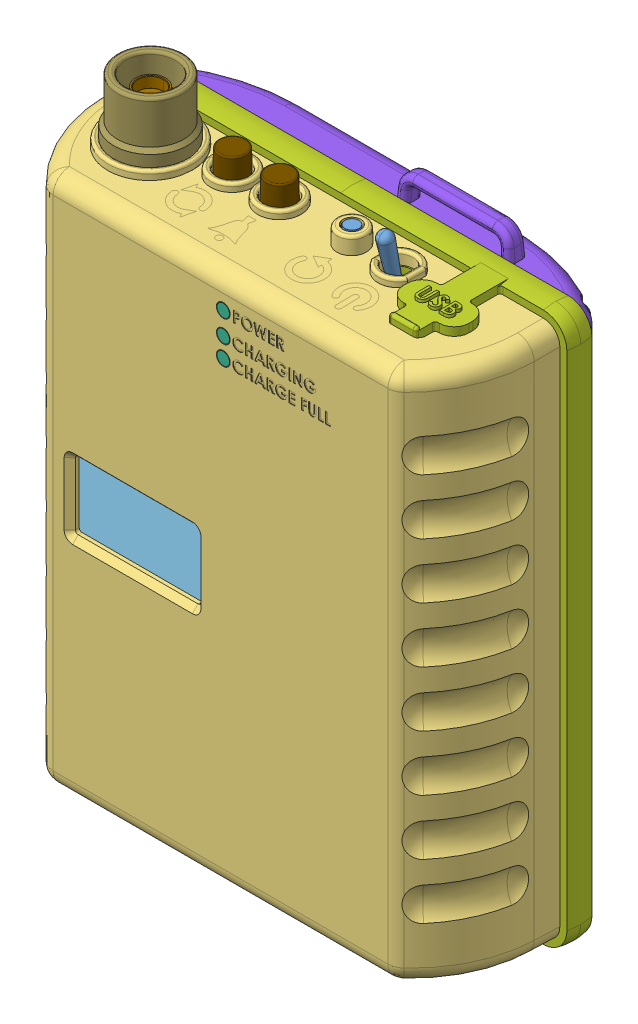
SolidWorks assembly TinyShuffle v.0, configuration Default. Lengths in mm.
Overall size (88.88 109.34 34.5).
53 component instances, 22 part files, 62 mates.
Components (placement in the parent):
- TinyShuffle PCBA v.0a-1: TinyShuffle PCBA v.0a [Default] at (-32.5 0 0) size (65 99.92 17.1)
- SWARM M138-1: SWARM M138 [Default] at (-32.6074 -0.0785 -0.4335) x (1 0 0) z (0 0 1) size (30 50.95 5.16)
- TinyShuffle TOP v.0-2: TinyShuffle TOP v.0 [Default] at origin size (87.38 99.33 23.32)
  - TinyShuffle TOP v.0-1: TinyShuffle TOP v.0 [Default] at origin size (87.38 99.33 23.15)
  - 94459A110_Heat-Set Inserts for Plastic m2X2.5-1: 94459A110_Heat-Set Inserts for Plastic m2X2.5 [94459A110] at (-36.2 89.5 -10.75) x (1 0 0) z (0 1 0) size (3.69 2.8 3.69)
  - 94459A110_Heat-Set Inserts for Plastic m2X2.5-2: 94459A110_Heat-Set Inserts for Plastic m2X2.5 [94459A110] at (36.2 89.5 -10.75) x (1 0 0) z (0 1 0) size (3.69 2.8 3.69)
  - 94459A110_Heat-Set Inserts for Plastic m2X2.5-3: 94459A110_Heat-Set Inserts for Plastic m2X2.5 [94459A110] at (36.2 44.25 -10.75) x (1 0 0) z (0 1 0) size (3.69 2.8 3.69)
  - 94459A110_Heat-Set Inserts for Plastic m2X2.5-4: 94459A110_Heat-Set Inserts for Plastic m2X2.5 [94459A110] at (36.2 -1 -10.75) x (1 0 0) z (0 1 0) size (3.69 2.8 3.69)
  - 94459A110_Heat-Set Inserts for Plastic m2X2.5-5: 94459A110_Heat-Set Inserts for Plastic m2X2.5 [94459A110] at (-36.2 -1 -10.75) x (1 0 0) z (0 1 0) size (3.69 2.8 3.69)
  - 94459A110_Heat-Set Inserts for Plastic m2X2.5-6: 94459A110_Heat-Set Inserts for Plastic m2X2.5 [94459A110] at (-36.2 44.25 -10.75) x (1 0 0) z (0 1 0) size (3.69 2.8 3.69)
  - TinyShuffle Display filter v.0-1: TinyShuffle Display filter v.0 [Default] at origin size (26.56 16.22 2.09)
  - BIVAR PLPC2-8MM-2: BIVAR PLPC2-8MM [Default] at (0.5 82.5 1.9) size (2.28 2.26 8.02)
  - BIVAR PLPC2-8MM-3: BIVAR PLPC2-8MM [Default] at (0.5 79 1.9) size (2.28 2.26 8.02)
  - BIVAR PLPC2-8MM-4: BIVAR PLPC2-8MM [Default] at (0.5 86.5 1.9) size (2.28 2.26 8.02)
  - 94459A110_Heat-Set Inserts for Plastic m2X2.5-7: 94459A110_Heat-Set Inserts for Plastic m2X2.5 [94459A110] at (29.5 75 2.5) x (1 0 0) z (0 1 0) size (3.69 2.8 3.69)
  - 94459A110_Heat-Set Inserts for Plastic m2X2.5-8: 94459A110_Heat-Set Inserts for Plastic m2X2.5 [94459A110] at (1 75 2.5) x (1 0 0) z (0 1 0) size (3.69 2.8 3.69)
  - 94459A110_Heat-Set Inserts for Plastic m2X2.5-9: 94459A110_Heat-Set Inserts for Plastic m2X2.5 [94459A110] at (-29.5 75 2.5) x (1 0 0) z (0 1 0) size (3.69 2.8 3.69)
  - 94459A110_Heat-Set Inserts for Plastic m2X2.5-10: 94459A110_Heat-Set Inserts for Plastic m2X2.5 [94459A110] at (-29.5 3 2.5) x (1 0 0) z (0 1 0) size (3.69 2.8 3.69)
  - 94459A110_Heat-Set Inserts for Plastic m2X2.5-11: 94459A110_Heat-Set Inserts for Plastic m2X2.5 [94459A110] at (29.5 3 2.5) x (1 0 0) z (0 1 0) size (3.69 2.8 3.69)
- TinyShuffle SHIM v.0-1: TinyShuffle SHIM v.0 [Default] at origin size (82 100.03 19.68)
- TinyShuffle BOT v.0-1: TinyShuffle BOT v.0 [Default] at origin size (79 101.5 24.59)
- SMA_CONNECTOR-1: SMA_CONNECTOR [Default] at (-26 101.6 -3.5) x (0 0 1) z (0 1 0) size (8.14 9.4 22.5)
- TYPE-C JACK-1: TYPE-C JACK [Default] at (26.205 88.375 -3.0876) x (0 0 1) z (0 1 0) size (6 10 35.27) (hidden)
- Swarm-1_4-wave-antenna-model-1: Swarm-1_4-wave-antenna-model [Default] at (-26 96.7375 -3.5) x (-1 0 0) z (0 1 0) size (11.04 11.04 215.14) (hidden)
- SMA_WASHER-1: SMA_WASHER [Default] at (-26 93 -3.5) x (1 0 0) z (0 -1 0) size (9 9 0.5)
- NT-SMA-N-1: NT-SMA-N [Default] at (-26 93.85 -3.5) x (0.997814 0 -0.066084) z (0 -1 0) size (9.24 8 1.7)
- TinyShuffle SMA SEAL v.0-1: TinyShuffle SMA SEAL v.0 [Default] at origin size (13.22 11.59 13.22)
- 92095A452_Button Head Hex Drive Screw M2x5-1: 92095A452_Button Head Hex Drive Screw M2x5 [92095A452] at (-27.3953 53.0669 5.935) size (3.5 3.5 6.52)
- 92095A452_Button Head Hex Drive Screw M2x5-2: 92095A452_Button Head Hex Drive Screw M2x5 [92095A452] at (-4.2953 53.0669 5.935) x (0.482092 -0.876121 0) z (0 0 1) size (3.5 3.5 6.52)
- 92095A452_Button Head Hex Drive Screw M2x5-3: 92095A452_Button Head Hex Drive Screw M2x5 [92095A452] at (-27.3953 29.5069 5.935) x (0.482092 -0.876121 0) z (0 0 1) size (3.5 3.5 6.52)
- 92095A452_Button Head Hex Drive Screw M2x5-4: 92095A452_Button Head Hex Drive Screw M2x5 [92095A452] at (-4.2953 29.5069 5.935) x (0.482092 -0.876121 0) z (0 0 1) size (3.5 3.5 6.52)
- 93475A195_18-8 Stainless Steel Washer M2X5-1: 93475A195_18-8 Stainless Steel Washer M2X5 [93475A195] at (29.5 75 -1.99) size (5 5 0.4)
- 93475A195_18-8 Stainless Steel Washer M2X5-2: 93475A195_18-8 Stainless Steel Washer M2X5 [93475A195] at (1 75 -1.99) size (5 5 0.4)
- 93475A195_18-8 Stainless Steel Washer M2X5-3: 93475A195_18-8 Stainless Steel Washer M2X5 [93475A195] at (-29.5 75 -1.99) size (5 5 0.4)
- 93475A195_18-8 Stainless Steel Washer M2X5-4: 93475A195_18-8 Stainless Steel Washer M2X5 [93475A195] at (-29.5 3 -1.99) size (5 5 0.4)
- 93475A195_18-8 Stainless Steel Washer M2X5-5: 93475A195_18-8 Stainless Steel Washer M2X5 [93475A195] at (29.5 3 -1.99) size (5 5 0.4)
- 92095A452_Button Head Hex Drive Screw M2x5-5: 92095A452_Button Head Hex Drive Screw M2x5 [92095A452] at (29.5 75 -3.29) x (1 0 0) z (0 0 -1) size (3.5 3.5 6.52)
- 92095A452_Button Head Hex Drive Screw M2x5-6: 92095A452_Button Head Hex Drive Screw M2x5 [92095A452] at (1 75 -3.29) x (1 0 0) z (0 0 -1) size (3.5 3.5 6.52)
- 92095A452_Button Head Hex Drive Screw M2x5-7: 92095A452_Button Head Hex Drive Screw M2x5 [92095A452] at (-29.5 75 -3.29) x (1 0 0) z (0 0 -1) size (3.5 3.5 6.52)
- 92095A452_Button Head Hex Drive Screw M2x5-8: 92095A452_Button Head Hex Drive Screw M2x5 [92095A452] at (-29.5 3 -3.29) x (1 0 0) z (0 0 -1) size (3.5 3.5 6.52)
- 92095A452_Button Head Hex Drive Screw M2x5-9: 92095A452_Button Head Hex Drive Screw M2x5 [92095A452] at (29.5 3 -3.29) x (1 0 0) z (0 0 -1) size (3.5 3.5 6.52)
- 92095A454_Button Head Hex Drive Screw M2X8-1: 92095A454_Button Head Hex Drive Screw M2X8 [92095A454] at (36.2 -1 -19.55) x (1 0 0) z (0 0 -1) size (3.5 3.5 9.53)
- 92095A454_Button Head Hex Drive Screw M2X8-2: 92095A454_Button Head Hex Drive Screw M2X8 [92095A454] at (36.2 44.25 -19.55) x (1 0 0) z (0 0 -1) size (3.5 3.5 9.53)
- 92095A454_Button Head Hex Drive Screw M2X8-3: 92095A454_Button Head Hex Drive Screw M2X8 [92095A454] at (36.2 89.5 -19.55) x (1 0 0) z (0 0 -1) size (3.5 3.5 9.53)
- 92095A454_Button Head Hex Drive Screw M2X8-4: 92095A454_Button Head Hex Drive Screw M2X8 [92095A454] at (-36.2 89.5 -19.55) x (1 0 0) z (0 0 -1) size (3.5 3.5 9.53)
- 92095A454_Button Head Hex Drive Screw M2X8-5: 92095A454_Button Head Hex Drive Screw M2X8 [92095A454] at (-36.2 44.25 -19.55) x (1 0 0) z (0 0 -1) size (3.5 3.5 9.53)
- 92095A454_Button Head Hex Drive Screw M2X8-6: 92095A454_Button Head Hex Drive Screw M2X8 [92095A454] at (-36.2 -1 -19.55) x (1 0 0) z (0 0 -1) size (3.5 3.5 9.53)
- 4035N11-1: 4035N11 [Default] at (-5 82.241 -22.209) x (-1 0 0) z (0 0 -1) size (12.7 12.7 0.38)
- W3908B0100-1: W3908B0100 [Default] at (15.25 63.7521 7.58) x (-1 0 0) z (0 0 -1) size (20 26.8 1.45)
- 800AC1BLKCAP-1: 800AC1BLKCAP [Default] at (-14 92.73 -6.27) x (1 0 0) z (0 0 1) size (5 5.03 5)
- 800AC1BLKCAP-2: 800AC1BLKCAP [Default] at (-5.5 92.73 -6.27) x (1 0 0) z (0 0 1) size (5 5.03 5)
- 353 Adafruit battery-1: 353 Adafruit battery [Default] at (-32.5 0.5 1) x (1 0 0) z (0 0 1) size (54 70 18)
- 3M 4026 FOAM .0625IN THICK-1: 3M 4026 FOAM .0625IN THICK [Default] at (-32.5 0.5 -20.59) x (-1 0 0) z (0 0 -1) size (35 65 1.59)
Mates (geometry in assembly coordinates):
- Coincident1: coincident: plane of assembly through (0 0 0) normal (0 0 1); plane of TinyShuffle PCBA v.0a-1 through (-32.5 0 0) normal (0 0 1); plane of assembly
- Symmetric1: symmetric: plane of assembly; plane of assembly; plane of TinyShuffle PCBA v.0a-1 through (-32.5 83.5 -1.59) normal (-1 0 0); plane of TinyShuffle PCBA v.0a-1 through (32.5 1 -1.59) normal (1 0 0); plane of assembly
- Coincident2: coincident: plane of assembly through (0 0 0) normal (0 1 0); plane of TinyShuffle PCBA v.0a-1 through (-32.5 0 0) normal (0 1 0); plane of assembly
- Parallel1: parallel aligned: plane of SMA_CONNECTOR-1 through (-27.5098 90.5 -0.7358) normal (0 0 1)
- Parallel2: parallel aligned: plane of SMA_CONNECTOR-1 through (-26 101.6 -3.5) normal (0 1 0)
- Distance1: distance = 3.5 mm aligned: plane of SMA_CONNECTOR-1 through (-26 101.6 -3.5) normal (0 0 1)
- Distance2: distance = 26 mm: plane of assembly through (0 0 0) normal (1 0 0); plane of assembly; plane of SMA_CONNECTOR-1 through (-26 101.6 -3.5) normal (1 0 0)
- Distance3: distance = 3.35 mm: plane of TinyShuffle PCBA v.0a-1 through (26.205 91.675 -3.0876) normal (0 1 0); plane of TYPE-C JACK-1 through (24.205 95.025 -3.0876) normal (0 -1 0)
- Width1: width: plane of TYPE-C JACK-1 through (24.205 110.025 -6.0876) normal (0 0 -1); plane of TinyShuffle PCBA v.0a-1 through (24.205 110.025 -0.0876) normal (0 0 1); plane of TYPE-C JACK-1 through (26.205 89.375 -4.3676) normal (0 0 1); plane of TinyShuffle PCBA v.0a-1 through (26.205 89.375 -1.8076) normal (0 0 -1)
- Distance4: distance = 26.205 mm: plane of assembly; plane of TYPE-C JACK-1 through (26.205 88.375 -3.0876) normal (1 0 0); point of assembly
- Concentric1: concentric: circle of SMA_CONNECTOR-1; circle of Swarm-1_4-wave-antenna-model-1
- Coincident3: coincident: plane of SMA_CONNECTOR-1 through (-26 99.5696 -3.5) normal (0 1 0); point of Swarm-1_4-wave-antenna-model-1
- Parallel3: parallel: plane of assembly through (0 0 0) normal (1 0 0); plane of Swarm-1_4-wave-antenna-model-1 through (-26 96.7375 -3.5) normal (-1 0 0); plane of assembly
- Concentric3: concentric anti-aligned: cone of TinyShuffle PCBA v.0a-1 through (-27.4 53.07 3.25) axis (0 0 -1); cylinder of pan head cross recess screw_iso-1 through (-27.4 53.07 31.635) axis (0 0 1) radius 2
- Coincident5: coincident anti-aligned: plane of TinyShuffle PCBA v.0a-1 through (-4.2953 53.0669 4.635) normal (0 0 1); plane of pan head cross recess screw_iso-1 through (-27.4 54.07 4.635) normal (0 0 -1)
- Concentric4: concentric: circle of TinyShuffle PCBA v.0-1; circle of 92095A452_Button Head Hex Drive Screw M2x5-1
- Coincident6: coincident: plane of TinyShuffle PCBA v.0a-1 through (-27.3953 53.0669 4.635) normal (0 0 1); circle of 92095A452_Button Head Hex Drive Screw M2x5-1
- Concentric5: concentric: circle of TinyShuffle PCBA v.0-1; circle of 92095A452_Button Head Hex Drive Screw M2x5-2
- Coincident7: coincident: plane of TinyShuffle PCBA v.0a-1 through (-4.2953 53.0669 4.635) normal (0 0 1); circle of 92095A452_Button Head Hex Drive Screw M2x5-2
- Coincident8: coincident: plane of TinyShuffle PCBA v.0a-1 through (-27.3953 29.5069 4.635) normal (0 0 1); circle of 92095A452_Button Head Hex Drive Screw M2x5-3
- Concentric6: concentric: circle of TinyShuffle PCBA v.0-1; circle of 92095A452_Button Head Hex Drive Screw M2x5-3
- Coincident9: coincident: plane of TinyShuffle PCBA v.0a-1 through (-4.2953 29.5069 4.635) normal (0 0 1); circle of 92095A452_Button Head Hex Drive Screw M2x5-4
- Concentric7: concentric: circle of TinyShuffle PCBA v.0-1; circle of 92095A452_Button Head Hex Drive Screw M2x5-4
- Concentric8: concentric aligned: circle of SMA_CONNECTOR-1; circle of SMA_WASHER-1
- Concentric9: concentric: circle of SMA_WASHER-1; circle of NT-SMA-N-1
- Coincident10: coincident: plane of SMA_WASHER-1 through (-26 93 -3.5) normal (0 1 0); plane of NT-SMA-N-1 through (-26 93 -3.5) normal (0 -1 0)
- ProfileCenter2: profile center: circle of 93475A195_18-8 Stainless Steel Washer M2X5-1; circle of TinyShuffle PCBA v.0-1
- ProfileCenter3: profile center: circle of 93475A195_18-8 Stainless Steel Washer M2X5-2; circle of TinyShuffle PCBA v.0-1
- ProfileCenter4: profile center: circle of 93475A195_18-8 Stainless Steel Washer M2X5-3; circle of TinyShuffle PCBA v.0-1
- ProfileCenter5: profile center: circle of 93475A195_18-8 Stainless Steel Washer M2X5-4; circle of TinyShuffle PCBA v.0-1
- ProfileCenter6: profile center: circle of 93475A195_18-8 Stainless Steel Washer M2X5-5; circle of TinyShuffle PCBA v.0-1
- ProfileCenter7: profile center: circle of 92095A452_Button Head Hex Drive Screw M2x5-5; circle of 93475A195_18-8 Stainless Steel Washer M2X5-1
- ProfileCenter8: profile center: circle of 92095A452_Button Head Hex Drive Screw M2x5-6; circle of 93475A195_18-8 Stainless Steel Washer M2X5-2
- ProfileCenter9: profile center: circle of 92095A452_Button Head Hex Drive Screw M2x5-7; circle of 93475A195_18-8 Stainless Steel Washer M2X5-3
- ProfileCenter10: profile center: circle of 92095A452_Button Head Hex Drive Screw M2x5-8; circle of 93475A195_18-8 Stainless Steel Washer M2X5-4
- ProfileCenter11: profile center: circle of 92095A452_Button Head Hex Drive Screw M2x5-9; circle of 93475A195_18-8 Stainless Steel Washer M2X5-5
- ProfileCenter12: profile center: circle of TinyShuffle BOT v.0-1; circle of 92095A454_Button Head Hex Drive Screw M2X8-1
- ProfileCenter13: profile center: circle of 92095A454_Button Head Hex Drive Screw M2X8-2; circle of TinyShuffle BOT v.0-1
- ProfileCenter14: profile center: circle of TinyShuffle BOT v.0-1; circle of 92095A454_Button Head Hex Drive Screw M2X8-3
- ProfileCenter15: profile center: circle of 92095A454_Button Head Hex Drive Screw M2X8-4; circle of TinyShuffle BOT v.0-1
- ProfileCenter16: profile center: circle of 92095A454_Button Head Hex Drive Screw M2X8-5; circle of TinyShuffle BOT v.0-1
- ProfileCenter17: profile center: circle of 92095A454_Button Head Hex Drive Screw M2X8-6; circle of TinyShuffle BOT v.0-1
- ProfileCenter18: profile center: circle of 4035N11-1; circle of TinyShuffle BOT v.0-1
- Coincident11: coincident: plane of TinyShuffle TOP v.0-2/TinyShuffle TOP v.0-1 through (31.3034 92.5 7.9) normal (0 0 -1); plane of W3908B0100-1 through (15.25 63.7521 7.9) normal (0 0 1)
- Parallel4: parallel aligned: line of TinyShuffle TOP v.0-2/TinyShuffle TOP v.0-1 through (30.1533 5.7617 7.9022) axis (0 1 0); line of W3908B0100-1 through (25.25 87.1736 7.9022) axis (-1 0 0)
- Parallel5: parallel: line of TinyShuffle TOP v.0-2/TinyShuffle TOP v.0-1 through (-33.5 90.5 -13.25) axis (1 0 0); line of W3908B0100-1 through (5.25 77.1521 7.58) axis (1 0 0)
- Distance5: distance = 12 mm: line of TinyShuffle TOP v.0-2/TinyShuffle TOP v.0-1 through (30.1556 89.1478 7.9) axis (-1 0 0); line of W3908B0100-1 through (5.25 77.1521 7.58) axis (1 0 0)
- Distance6: distance = 14.25 mm: plane of W3908B0100-1 through (15.25 63.7521 7.58) normal (-1 0 0); unknown of ?
- Coincident12: coincident: plane of TinyShuffle PCBA v.0a-1 through (-12.603 95.33 -7.667) normal (0 1 0); plane of 800AC1BLKCAP-1 through (-14 95.33 -5.62) normal (0 -1 0)
- Concentric10: concentric: circle of TinyShuffle PCBA v.0a-1; cone of 800AC1BLKCAP-1 through (-14 96.76 -6.27) axis (0 1 0)
- Coincident13: coincident: plane of TinyShuffle PCBA v.0a-1 through (-4.103 95.33 -7.667) normal (0 1 0); plane of 800AC1BLKCAP-2 through (-5.5 95.33 -5.62) normal (0 -1 0)
- Concentric11: concentric: circle of TinyShuffle PCBA v.0a-1; cone of 800AC1BLKCAP-2 through (-5.5 96.76 -6.27) axis (0 1 0)
- Concentric12: concentric: circle of TinyShuffle PCBA v.0a-1; circle of SWARM M138-1
- Width2: width: plane of TinyShuffle PCBA v.0a-1 through (0.2088 62.6755 1.1) normal (0 0 1); plane of SWARM M138-1 through (27.6088 66.7755 2.5) normal (0 0 -1); plane of TinyShuffle PCBA v.0a-1 through (27.5588 15.7365 1.3345) normal (0 0 -1); plane of SWARM M138-1 through (27.5588 15.7365 2.2655) normal (0 0 1)
- Concentric13: concentric: circle of TinyShuffle PCBA v.0a-1; circle of SWARM M138-1
- Distance7: distance = 1 mm: plane of 353 Adafruit battery-1 through (0 35.5 -2.59) normal (0 0 1); plane of TinyShuffle PCBA v.0a-1 through (-32.5 1 -1.59) normal (0 0 -1)
- Symmetric2: symmetric: cylinder of assembly; cylinder of assembly; cylinder of 353 Adafruit battery-1 through (-18 18 -11.59) axis (0 1 0) radius 9; cylinder of 353 Adafruit battery-1 through (18 53 -11.59) axis (0 -1 0) radius 9; plane of assembly
- Distance8: distance = 0.5 mm: plane of 353 Adafruit battery-1 through (27 0.5 -2.59) normal (0 -1 0); plane of TinyShuffle PCBA v.0a-1 through (-31.5 0 -1.59) normal (0 -1 0)
- InPlace1: in place: plane of 353 Adafruit battery-1 through (0 35.5 -20.59) normal (0 0 -1); plane of ? through (0 0 -20.59) normal (0 0 -1); moOrthogonalPlaneRef_w of 353 Adafruit battery-1 through (0 35.5 -20.59) normal (0 0 -1); plane of ? through (0 0 -20.59) normal (0 1 0); plane of 353 Adafruit battery-1 through (0 35.5 -20.59) normal (0 0 -1); plane of ? through (0 0 -20.59) normal (-1 0 0); plane of 353 Adafruit battery-1 through (0 35.5 -20.59) normal (0 0 -1); unknown of 3M 4026 FOAM .0625IN THICK-1
- Coincident14: coincident: plane of ?; plane of ?
- Coincident15: coincident: moOrthogonalPlaneRef_w of 353 Adafruit battery-1 through (-32.5 0.5 -20.59) normal (0 1 0); plane of Part1^TinyShuffle v.0-1 through (-32.5 0.5 -20.59) normal (0 1 0)
- Coincident16: coincident: moOrthogonalPlaneRef_w of 353 Adafruit battery-1 through (-32.5 0.5 -20.59) normal (1 0 0); plane of Part1^TinyShuffle v.0-1 through (-32.5 0.5 -20.59) normal (-1 0 0)
